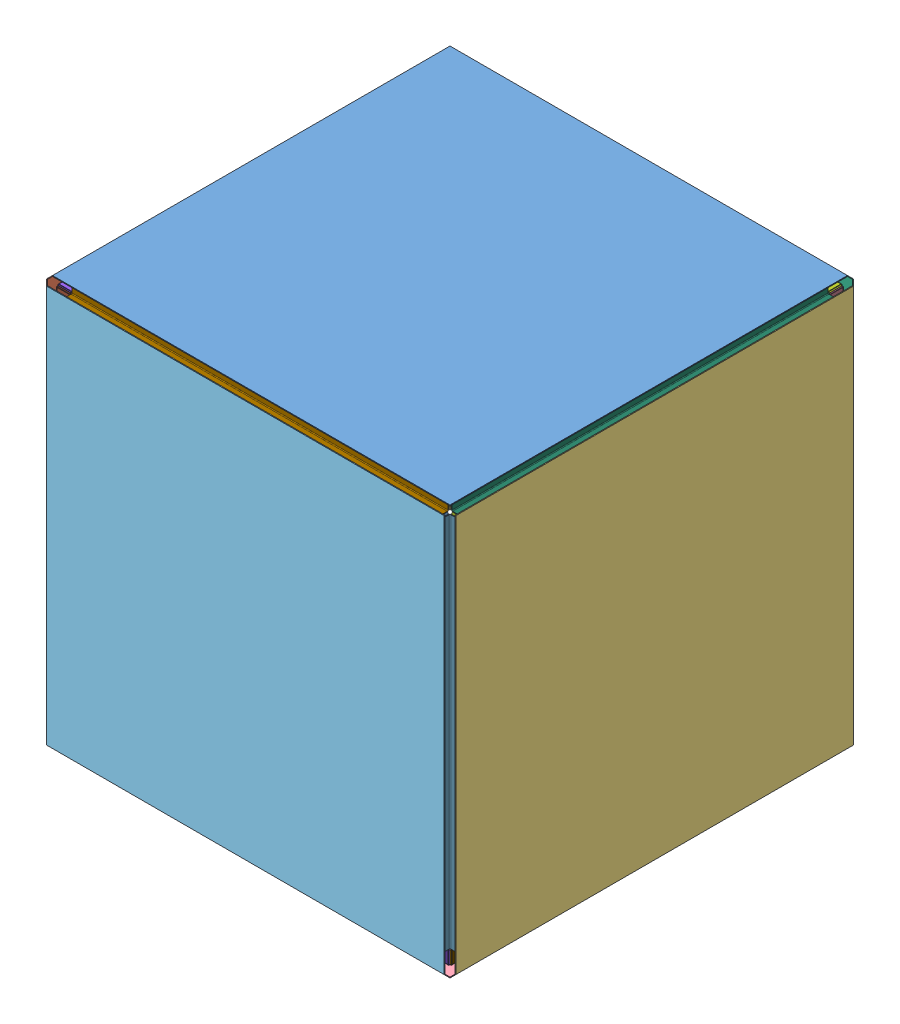
SolidWorks assembly cube_30, configuration cube30. Lengths in mm.
Overall size (747.39 747.39 747.39).
30 component instances, 30 part files, 93 mates.
Components (placement in the parent):
- pr^cube_30-28: pr^cube_30 [cube01] x (-1 0 0) z (0 0 1) size (725.17 1.59 725.17) (virtual)
- pg^cube_30-20: pg^cube_30 [cube01] x (0 -1 0) z (0 0 1) size (725.17 1.59 725.17) (virtual)
- po^cube_30-22: po^cube_30 [cube01] x (0 1 0) z (0 0 1) size (725.17 1.59 725.17) (virtual)
- py^cube_30-21: py^cube_30 [cube01] at origin size (725.17 1.59 725.17) (virtual)
- pc^cube_30-18: pc^cube_30 [cube01] x (-1 0 0) z (0 -1 0) size (725.17 1.59 725.17) (virtual)
- pb^cube_30-21: pb^cube_30 [cube01] x (-1 0 0) z (0 1 0) size (725.17 1.59 725.17) (virtual)
- br1^cube_30-49: br1^cube_30 [Default] at (0 346.71 -346.71) x (0 0 1) z (-1 0 0) size (50.8 50.8 686.31) (virtual)
- br2^cube_30-61: br2^cube_30 [Default] at (-346.71 346.71 0) size (50.8 50.8 686.31) (virtual)
- br3^cube_30-46: br3^cube_30 [Default] at (0 346.71 346.71) x (0 0 -1) z (1 0 0) size (50.8 50.8 686.31) (virtual)
- bg1^cube_30-47: bg1^cube_30 [Default] at (-346.71 -346.71 0) x (0 1 0) z (0 0 1) size (50.8 50.8 686.31) (virtual)
- bg2^cube_30-44: bg2^cube_30 [Default] at (-346.71 0 346.71) x (0 0 -1) z (0 1 0) size (50.8 50.8 686.31) (virtual)
- bg3^cube_30-40: bg3^cube_30 [Default] at (-346.71 0 -346.71) x (0 0 1) z (0 -1 0) size (50.8 50.8 686.31) (virtual)
- bo1^cube_30-42: bo1^cube_30 [Default] at (346.71 0 -346.71) x (0 0 1) z (0 1 0) size (50.8 50.8 686.31) (virtual)
- bo2^cube_30-46: bo2^cube_30 [Default] at (346.71 0 346.71) x (0 0 -1) z (0 -1 0) size (50.8 50.8 686.31) (virtual)
- bo3^cube_30-62: bo3^cube_30 [Default] at (346.71 346.71 0) x (0 -1 0) z (0 0 1) size (50.8 50.8 686.31) (virtual)
- by1^cube_30-41: by1^cube_30 [Default] at (0 -346.71 -346.71) x (0 0 1) z (1 0 0) size (50.8 50.8 686.31) (virtual)
- by2^cube_30-45: by2^cube_30 [Default] at (0 -346.71 346.71) x (0 0 -1) z (-1 0 0) size (50.8 50.8 686.31) (virtual)
- by3^cube_30-48: by3^cube_30 [Default] at (346.71 -346.71 0) x (-1 0 0) z (0 0 1) size (50.8 50.8 686.31) (virtual)
- dr1^cube_30-55: dr1^cube_30 [cube01] at (-371.5046 372.11 0) x (0 -1 0) z (0 0 1) size (26.01 26.01 744.23) (hidden, virtual)
- dr2^cube_30-37: dr2^cube_30 [cube01] at (0 372.11 371.5046) x (0 -1 0) z (1 0 0) size (26.01 26.01 744.23) (hidden, virtual)
- dr3^cube_30-33: dr3^cube_30 [cube01] at (0 372.11 -371.5046) x (0 -1 0) z (-1 0 0) size (26.01 26.01 744.23) (hidden, virtual)
- dg1^cube_30-38: dg1^cube_30 [cube01] at (-372.11 0 371.5046) x (1 0 0) z (0 1 0) size (26.01 26.01 744.23) (hidden, virtual)
- dg2^cube_30-41: dg2^cube_30 [cube01] at (-372.11 -371.5046 0) size (26.01 26.01 744.23) (hidden, virtual)
- dg3^cube_30-34: dg3^cube_30 [cube01] at (-372.11 0 -371.5046) x (1 0 0) z (0 -1 0) size (26.01 26.01 744.23) (hidden, virtual)
- do3^cube_30-47: do3^cube_30 [cube01] at (372.11 371.5046 0) x (-1 0 0) z (0 0 1) size (26.01 26.01 744.23) (hidden, virtual)
- do1^cube_30-36: do1^cube_30 [cube01] at (372.11 0 -371.5046) x (-1 0 0) z (0 1 0) size (26.01 26.01 744.23) (hidden, virtual)
- do2^cube_30-40: do2^cube_30 [cube01] at (372.11 0 371.5046) x (-1 0 0) z (0 -1 0) size (26.01 26.01 744.23) (hidden, virtual)
- dy1^cube_30-35: dy1^cube_30 [cube01] at (0 -372.11 -371.5046) x (0 1 0) z (1 0 0) size (26.01 26.01 744.23) (hidden, virtual)
- dy2^cube_30-39: dy2^cube_30 [cube01] at (0 -372.11 371.5046) x (0 1 0) z (-1 0 0) size (26.01 26.01 744.23) (hidden, virtual)
- dy3^cube_30-42: dy3^cube_30 [cube01] at (371.5046 -372.11 0) x (0 1 0) z (0 0 1) size (26.01 26.01 744.23) (hidden, virtual)
Mates (geometry in assembly coordinates):
- Coincident1: coincident anti-aligned: plane of pr^cube_30-28 through (362.585 372.11 -362.585) normal (0 -1 0); plane of br1^cube_30-49 through (-343.154 372.11 -346.71) normal (0 1 0)
- Coincident2: coincident anti-aligned: plane of pr^cube_30-28 through (362.585 372.11 -362.585) normal (0 -1 0); plane of br2^cube_30-61 through (-346.71 372.11 343.154) normal (0 1 0)
- Coincident3: coincident anti-aligned: plane of pr^cube_30-28 through (362.585 372.11 -362.585) normal (0 -1 0); plane of br3^cube_30-46 through (343.154 372.11 346.71) normal (0 1 0)
- Coincident4: coincident anti-aligned: plane of pr^cube_30-28 through (362.585 372.11 -362.585) normal (0 -1 0); plane of bo3^cube_30-62 through (346.71 372.11 343.154) normal (0 1 0)
- Coincident5: coincident anti-aligned: plane of pr^cube_30-28 through (362.585 372.11 -362.585) normal (0 -1 0); plane of dr3^cube_30-33 through (0 372.11 -743.6146) normal (0 1 0)
- Coincident6: coincident anti-aligned: plane of pr^cube_30-28 through (362.585 372.11 -362.585) normal (0 -1 0); plane of dr1^cube_30-55 through (-743.6146 372.11 0) normal (0 1 0)
- Coincident7: coincident anti-aligned: plane of pr^cube_30-28 through (362.585 372.11 -362.585) normal (0 -1 0); plane of do3^cube_30-47 through (-0.6054 372.11 0) normal (0 1 0)
- Coincident8: coincident anti-aligned: plane of pr^cube_30-28 through (362.585 372.11 -362.585) normal (0 -1 0); plane of dr2^cube_30-37 through (0 372.11 743.6146) normal (0 1 0)
- Coincident34: coincident anti-aligned: plane of pb^cube_30-21 through (362.585 -362.585 -372.11) normal (0 0 1); plane of by1^cube_30-41 through (343.154 -346.71 -372.11) normal (0 0 -1)
- Coincident35: coincident anti-aligned: plane of pb^cube_30-21 through (362.585 -362.585 -372.11) normal (0 0 1); plane of bo1^cube_30-42 through (346.71 343.154 -372.11) normal (0 0 -1)
- Coincident36: coincident anti-aligned: plane of pb^cube_30-21 through (362.585 -362.585 -372.11) normal (0 0 1); plane of br1^cube_30-49 through (-343.154 346.71 -372.11) normal (0 0 -1)
- Coincident37: coincident anti-aligned: plane of pb^cube_30-21 through (362.585 -362.585 -372.11) normal (0 0 1); plane of bg3^cube_30-40 through (-346.71 -343.154 -372.11) normal (0 0 -1)
- Coincident38: coincident anti-aligned: plane of pb^cube_30-21 through (362.585 -362.585 -372.11) normal (0 0 1); plane of dg3^cube_30-34 through (0.6054 0 -372.11) normal (0 0 -1)
- Coincident39: coincident anti-aligned: plane of pb^cube_30-21 through (362.585 -362.585 -372.11) normal (0 0 1); plane of dr3^cube_30-33 through (0 -0.6054 -372.11) normal (0 0 -1)
- Coincident40: coincident anti-aligned: plane of pb^cube_30-21 through (362.585 -362.585 -372.11) normal (0 0 1); plane of do1^cube_30-36 through (-0.6054 0 -372.11) normal (0 0 -1)
- Coincident41: coincident anti-aligned: plane of pb^cube_30-21 through (362.585 -362.585 -372.11) normal (0 0 1); plane of dy1^cube_30-35 through (0 0.6054 -372.11) normal (0 0 -1)
- Coincident42: coincident anti-aligned: plane of pc^cube_30-18 through (362.585 362.585 372.11) normal (0 0 -1); plane of bo2^cube_30-46 through (346.71 -343.154 372.11) normal (0 0 1)
- Coincident43: coincident anti-aligned: plane of pc^cube_30-18 through (362.585 362.585 372.11) normal (0 0 -1); plane of br3^cube_30-46 through (343.154 346.71 372.11) normal (0 0 1)
- Coincident44: coincident anti-aligned: plane of pc^cube_30-18 through (362.585 362.585 372.11) normal (0 0 -1); plane of bg2^cube_30-44 through (-346.71 343.154 372.11) normal (0 0 1)
- Coincident45: coincident anti-aligned: plane of pc^cube_30-18 through (362.585 362.585 372.11) normal (0 0 -1); plane of by2^cube_30-45 through (-343.154 -346.71 372.11) normal (0 0 1)
- Coincident46: coincident anti-aligned: plane of pc^cube_30-18 through (362.585 362.585 372.11) normal (0 0 -1); plane of do2^cube_30-40 through (-0.6054 0 372.11) normal (0 0 1)
- Coincident47: coincident anti-aligned: plane of pc^cube_30-18 through (362.585 362.585 372.11) normal (0 0 -1); plane of dy2^cube_30-39 through (0 0.6054 372.11) normal (0 0 1)
- Coincident48: coincident anti-aligned: plane of pc^cube_30-18 through (362.585 362.585 372.11) normal (0 0 -1); plane of dg1^cube_30-38 through (0.6054 0 372.11) normal (0 0 1)
- Coincident49: coincident anti-aligned: plane of pc^cube_30-18 through (362.585 362.585 372.11) normal (0 0 -1); plane of dr2^cube_30-37 through (0 -0.6054 372.11) normal (0 0 1)
- Coincident50: coincident anti-aligned: plane of pg^cube_30-20 through (-372.11 362.585 -362.585) normal (1 0 0); plane of bg3^cube_30-40 through (-372.11 -343.154 -346.71) normal (-1 0 0)
- Coincident51: coincident anti-aligned: plane of pg^cube_30-20 through (-372.11 362.585 -362.585) normal (1 0 0); plane of bg1^cube_30-47 through (-372.11 -346.71 343.154) normal (-1 0 0)
- Coincident52: coincident anti-aligned: plane of pg^cube_30-20 through (-372.11 362.585 -362.585) normal (1 0 0); plane of bg2^cube_30-44 through (-372.11 343.154 346.71) normal (-1 0 0)
- Coincident53: coincident anti-aligned: plane of pg^cube_30-20 through (-372.11 362.585 -362.585) normal (1 0 0); plane of dr1^cube_30-55 through (-372.11 -0.6054 0) normal (-1 0 0)
- Coincident54: coincident anti-aligned: plane of pg^cube_30-20 through (-372.11 362.585 -362.585) normal (1 0 0); plane of dg3^cube_30-34 through (-372.11 0 -743.6146) normal (-1 0 0)
- Coincident55: coincident anti-aligned: plane of pg^cube_30-20 through (-372.11 362.585 -362.585) normal (1 0 0); plane of dg2^cube_30-41 through (-372.11 -743.6146 0) normal (-1 0 0)
- Coincident56: coincident anti-aligned: plane of pg^cube_30-20 through (-372.11 362.585 -362.585) normal (1 0 0); plane of dg1^cube_30-38 through (-372.11 0 743.6146) normal (-1 0 0)
- Coincident99: coincident anti-aligned: plane of pg^cube_30-20 through (-372.11 362.585 -362.585) normal (1 0 0); plane of br2^cube_30-61 through (-372.11 346.71 343.154) normal (-1 0 0)
- Coincident57: coincident anti-aligned: plane of py^cube_30-21 through (-362.585 -372.11 -362.585) normal (0 1 0); plane of by3^cube_30-48 through (346.71 -372.11 343.154) normal (0 -1 0)
- Coincident58: coincident anti-aligned: plane of py^cube_30-21 through (-362.585 -372.11 -362.585) normal (0 1 0); plane of by2^cube_30-45 through (-343.154 -372.11 346.71) normal (0 -1 0)
- Coincident59: coincident anti-aligned: plane of py^cube_30-21 through (-362.585 -372.11 -362.585) normal (0 1 0); plane of bg1^cube_30-47 through (-346.71 -372.11 343.154) normal (0 -1 0)
- Coincident60: coincident anti-aligned: plane of py^cube_30-21 through (-362.585 -372.11 -362.585) normal (0 1 0); plane of by1^cube_30-41 through (343.154 -372.11 -346.71) normal (0 -1 0)
- Coincident61: coincident anti-aligned: plane of py^cube_30-21 through (-362.585 -372.11 -362.585) normal (0 1 0); plane of dy3^cube_30-42 through (743.6146 -372.11 0) normal (0 -1 0)
- Coincident62: coincident anti-aligned: plane of py^cube_30-21 through (-362.585 -372.11 -362.585) normal (0 1 0); plane of dy2^cube_30-39 through (0 -372.11 743.6146) normal (0 -1 0)
- Coincident63: coincident anti-aligned: plane of py^cube_30-21 through (-362.585 -372.11 -362.585) normal (0 1 0); plane of dg2^cube_30-41 through (0.6054 -372.11 0) normal (0 -1 0)
- Coincident64: coincident anti-aligned: plane of py^cube_30-21 through (-362.585 -372.11 -362.585) normal (0 1 0); plane of dy1^cube_30-35 through (0 -372.11 -743.6146) normal (0 -1 0)
- Coincident65: coincident anti-aligned: plane of po^cube_30-22 through (372.11 -362.585 -362.585) normal (-1 0 0); plane of bo1^cube_30-42 through (372.11 343.154 -346.71) normal (1 0 0)
- Coincident66: coincident anti-aligned: plane of po^cube_30-22 through (372.11 -362.585 -362.585) normal (-1 0 0); plane of by3^cube_30-48 through (372.11 -346.71 343.154) normal (1 0 0)
- Coincident67: coincident anti-aligned: plane of po^cube_30-22 through (372.11 -362.585 -362.585) normal (-1 0 0); plane of bo2^cube_30-46 through (372.11 -343.154 346.71) normal (1 0 0)
- Coincident68: coincident anti-aligned: plane of po^cube_30-22 through (372.11 -362.585 -362.585) normal (-1 0 0); plane of bo3^cube_30-62 through (372.11 346.71 343.154) normal (1 0 0)
- Coincident69: coincident anti-aligned: plane of po^cube_30-22 through (372.11 -362.585 -362.585) normal (-1 0 0); plane of do2^cube_30-40 through (372.11 0 743.6146) normal (1 0 0)
- Coincident70: coincident anti-aligned: plane of po^cube_30-22 through (372.11 -362.585 -362.585) normal (-1 0 0); plane of do3^cube_30-47 through (372.11 743.6146 0) normal (1 0 0)
- Coincident71: coincident anti-aligned: plane of po^cube_30-22 through (372.11 -362.585 -362.585) normal (-1 0 0); plane of do1^cube_30-36 through (372.11 0 -743.6146) normal (1 0 0)
- Coincident72: coincident anti-aligned: plane of po^cube_30-22 through (372.11 -362.585 -362.585) normal (-1 0 0); plane of dy3^cube_30-42 through (372.11 0.6054 0) normal (1 0 0)
- Coincident73: coincident aligned: plane of assembly through (0 0 0) normal (0 0 1); plane of dy3^cube_30-42 through (371.5046 -372.11 0) normal (0 0 1)
- Coincident74: coincident aligned: plane of assembly through (0 0 0) normal (0 0 1); plane of by3^cube_30-48 through (346.71 -346.71 0) normal (0 0 1)
- Coincident75: coincident aligned: plane of assembly through (0 0 0) normal (0 0 1); plane of bo3^cube_30-62 through (346.71 346.71 0) normal (0 0 1)
- Coincident76: coincident aligned: plane of assembly through (0 0 0) normal (0 0 1); plane of do3^cube_30-47 through (372.11 371.5046 0) normal (0 0 1)
- Coincident77: coincident aligned: plane of assembly through (0 0 0) normal (0 0 1); plane of dg2^cube_30-41 through (-372.11 -371.5046 0) normal (0 0 1)
- Coincident78: coincident aligned: plane of assembly through (0 0 0) normal (0 0 1); plane of bg1^cube_30-47 through (-346.71 -346.71 0) normal (0 0 1)
- Coincident79: coincident aligned: plane of assembly through (0 0 0) normal (0 0 1); plane of dr1^cube_30-55 through (-371.5046 372.11 0) normal (0 0 1)
- Coincident80: coincident aligned: plane of assembly through (0 0 0) normal (0 0 1); plane of br2^cube_30-61 through (-346.71 346.71 0) normal (0 0 1)
- Coincident81: coincident aligned: plane of assembly through (0 0 0) normal (0 1 0); plane of bo1^cube_30-42 through (346.71 0 -346.71) normal (0 1 0)
- Coincident82: coincident aligned: plane of assembly through (0 0 0) normal (0 1 0); plane of py^cube_30-21 through (0 0 0) normal (0 1 0)
- Coincident83: coincident aligned: plane of assembly through (0 0 0) normal (0 1 0); plane of do1^cube_30-36 through (372.11 0 -371.5046) normal (0 1 0)
- Coincident84: coincident anti-aligned: plane of assembly through (0 0 0) normal (0 1 0); plane of bg3^cube_30-40 through (-346.71 0 -346.71) normal (0 -1 0)
- Coincident85: coincident anti-aligned: plane of assembly through (0 0 0) normal (0 1 0); plane of dg3^cube_30-34 through (-372.11 0 -371.5046) normal (0 -1 0)
- Coincident86: coincident aligned: plane of assembly through (0 0 0) normal (0 1 0); plane of dg1^cube_30-38 through (-372.11 0 371.5046) normal (0 1 0)
- Coincident87: coincident aligned: plane of assembly through (0 0 0) normal (0 1 0); plane of bg2^cube_30-44 through (-346.71 0 346.71) normal (0 1 0)
- Coincident88: coincident anti-aligned: plane of assembly through (0 0 0) normal (0 1 0); plane of bo2^cube_30-46 through (346.71 0 346.71) normal (0 -1 0)
- Coincident89: coincident anti-aligned: plane of assembly through (0 0 0) normal (0 1 0); plane of do2^cube_30-40 through (372.11 0 371.5046) normal (0 -1 0)
- Coincident90: coincident anti-aligned: plane of assembly through (0 0 0) normal (1 0 0); plane of by2^cube_30-45 through (0 -346.71 346.71) normal (-1 0 0)
- Coincident91: coincident anti-aligned: plane of assembly through (0 0 0) normal (1 0 0); plane of dy2^cube_30-39 through (0 -372.11 371.5046) normal (-1 0 0)
- Coincident92: coincident aligned: plane of assembly through (0 0 0) normal (1 0 0); plane of pg^cube_30-20
- Coincident93: coincident aligned: plane of assembly through (0 0 0) normal (1 0 0); plane of dr2^cube_30-37 through (0 372.11 371.5046) normal (1 0 0)
- Coincident94: coincident aligned: plane of assembly through (0 0 0) normal (1 0 0); plane of br3^cube_30-46 through (0 346.71 346.71) normal (1 0 0)
- Coincident95: coincident anti-aligned: plane of assembly through (0 0 0) normal (1 0 0); plane of dr3^cube_30-33 through (0 372.11 -371.5046) normal (-1 0 0)
- Coincident96: coincident anti-aligned: plane of assembly through (0 0 0) normal (1 0 0); plane of br1^cube_30-49 through (0 346.71 -346.71) normal (-1 0 0)
- Coincident97: coincident aligned: plane of assembly through (0 0 0) normal (1 0 0); plane of by1^cube_30-41 through (0 -346.71 -346.71) normal (1 0 0)
- Coincident98: coincident aligned: plane of assembly through (0 0 0) normal (1 0 0); plane of dy1^cube_30-35 through (0 -372.11 -371.5046) normal (1 0 0)
- Coincident100: coincident anti-aligned: plane of pr^cube_30-28; plane of assembly through (0 0 0) normal (1 0 0)
- Coincident101: coincident aligned: plane of pr^cube_30-28 through (0 0 0) normal (0 0 1); plane of assembly through (0 0 0) normal (0 0 1)
- Coincident102: coincident anti-aligned: plane of pr^cube_30-28; plane of assembly through (0 0 0) normal (0 1 0)
- Coincident106: coincident anti-aligned: plane of pg^cube_30-20; plane of assembly through (0 0 0) normal (0 1 0)
- Coincident107: coincident aligned: plane of pg^cube_30-20; plane of assembly through (0 0 0) normal (1 0 0)
- Coincident108: coincident aligned: plane of pg^cube_30-20 through (0 0 0) normal (0 0 1); plane of assembly through (0 0 0) normal (0 0 1)
- Coincident109: coincident aligned: plane of py^cube_30-21 through (0 0 0) normal (0 0 1); plane of assembly through (0 0 0) normal (0 0 1)
- Coincident110: coincident aligned: plane of py^cube_30-21 through (0 0 0) normal (0 1 0); plane of assembly through (0 0 0) normal (0 1 0)
- Coincident111: coincident aligned: plane of py^cube_30-21 through (0 0 0) normal (1 0 0); plane of assembly through (0 0 0) normal (1 0 0)
- Coincident112: coincident aligned: plane of po^cube_30-22 through (0 0 0) normal (0 0 1); plane of assembly through (0 0 0) normal (0 0 1)
- Coincident113: coincident anti-aligned: plane of po^cube_30-22; plane of assembly through (0 0 0) normal (1 0 0)
- Coincident114: coincident aligned: plane of po^cube_30-22; plane of assembly through (0 0 0) normal (0 1 0)
- Coincident115: coincident anti-aligned: plane of pc^cube_30-18 through (0 0 0) normal (0 -1 0); plane of assembly through (0 0 0) normal (0 1 0)
- Coincident116: coincident anti-aligned: plane of pc^cube_30-18; plane of assembly through (0 0 0) normal (0 0 1)
- Coincident117: coincident anti-aligned: plane of pc^cube_30-18; plane of assembly through (0 0 0) normal (1 0 0)
- Coincident118: coincident aligned: plane of pb^cube_30-21 through (0 0 0) normal (0 1 0); plane of assembly through (0 0 0) normal (0 1 0)
- Coincident119: coincident aligned: plane of pb^cube_30-21; plane of assembly through (0 0 0) normal (0 0 1)
- Coincident120: coincident anti-aligned: line of pb^cube_30-21 through (0.8731 -0.8731 0) axis (0 0 -1); sketch_entity of pr^cube_30-28; plane of pb^cube_30-21 through (362.585 -362.585 -373.6975) normal (0 0 -1); plane of py^cube_30-21 through (-362.585 -373.6975 -362.585) normal (0 -1 0)
- cyan_cut: unknown: unknown of pc^cube_30-18; plane of pc^cube_30-18 through (362.585 362.585 373.6975) normal (0 0 1); plane of pg^cube_30-20 through (-373.6975 362.585 -362.585) normal (-1 0 0); plane of po^cube_30-22 through (373.6975 -362.585 -362.585) normal (1 0 0)
